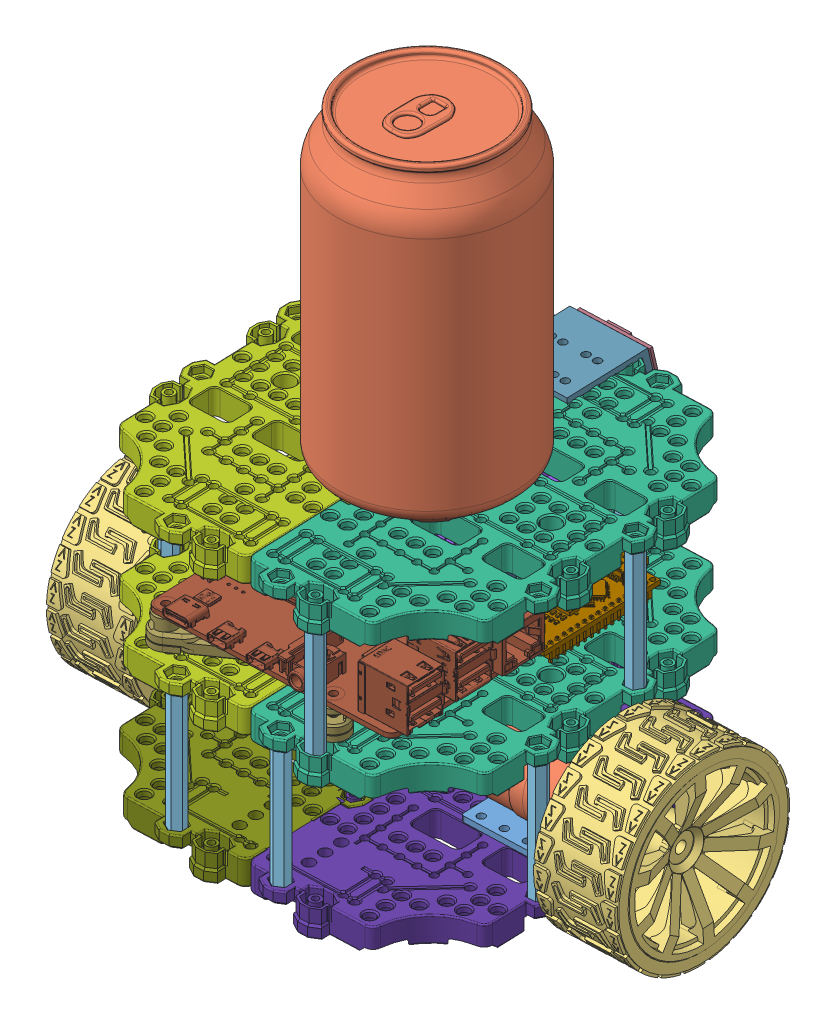
SolidWorks assembly BumperBotConveyor, configuration Default. Lengths in mm.
Overall size (200.73 230.35 157.69).
44 component instances, 20 part files, 117 mates.
Components (placement in the parent):
- motor_support-1: motor_support [Default] at (-39.885 107.5277 104.4569) x (-0.035505 0 -0.999369) z (0.999369 0 -0.035505) size (28 29 41)
- motor_support-2: motor_support [Default] at (97.5755 107.5277 99.5732) x (0.035505 0 0.999369) z (-0.999369 0 0.035505) size (28 29 41)
- JGA25-370-1: JGA25-370 [Default] at (52.3299 107.5277 101.1807) x (0.999369 0 -0.035505) z (0 -1 0) size (70.5 25.2 25.2)
- JGA25-370-2: JGA25-370 [Default] at (5.3607 107.5277 102.8494) x (-0.999369 0 0.035505) z (0 -1 0) size (70.5 25.2 25.2)
- wheel-1: wheel [Default] at (-18.4133 64.9311 67.753) x (0.033104 -0.361489 0.931789) z (-0.999369 0 0.035505) size (65.01 65.01 29)
- wheel_motor_adapter-1: wheel_motor_adapter [Default] at (-52.3777 107.532 104.885) x (0.034231 -0.265538 0.963493) z (-0.999369 0 0.035505) size (13.7 12 18.23)
- wheel-2: wheel [Default] at (76.6746 127.5563 152.3432) x (0.001314 -0.999315 0.036975) z (0.999369 0 -0.035505) size (65.01 65.01 29)
- wheel_motor_adapter-2: wheel_motor_adapter [Default] at (110.0677 107.5439 99.1304) x (-0.002274 -0.997947 -0.064012) z (0.999369 0 -0.035505) size (13.7 12 18.23)
- SUPPORT_HEX_M3_0XL45_FF-1: SUPPORT_HEX_M3_0XL45_FF [Default] at (50.5578 90.0277 37.2033) x (-0.5 0 0.866025) z (-0.866025 0 -0.5) size (5 45 5.77)
- SUPPORT_HEX_M3_0XL45_FF-6: SUPPORT_HEX_M3_0XL45_FF [Default] at (7.1327 90.0277 166.8268) x (0.255141 0 -0.966904) z (0.966904 0 0.255141) size (5 45 5.77)
- waffle_front_plate-3: waffle_front_plate [Default] at (28.8453 139.5277 102.0151) x (0.999369 0 -0.035505) z (0.035505 0 0.999369) size (73.55 9.85 137.55)
- waffle_rear_plate-2: waffle_rear_plate [Default] at (28.8453 139.5277 102.0151) x (-0.999369 0 0.035505) z (-0.035505 0 -0.999369) size (73.55 9.85 137.55)
- SUPPORT_HEX_M3_0XL45_FF-7: SUPPORT_HEX_M3_0XL45_FF [Default] at (2.588 87.5277 38.9075) x (0 0 -1) z (1 0 0) size (5 45 5.77)
- SUPPORT_HEX_M3_0XL45_FF-17: SUPPORT_HEX_M3_0XL45_FF [Default] at (-35.9665 135.0277 80.3025) x (0.866025 0 0.5) z (0.5 0 -0.866025) size (5 45 5.77)
- SUPPORT_HEX_M3_0XL45_FF-18: SUPPORT_HEX_M3_0XL45_FF [Default] at (93.657 135.0277 123.7276) x (0.866025 0 0.5) z (0.5 0 -0.866025) size (5 45 5.77)
- L298N-2: L298N [Default] at (11.4909 149.5277 70.3617) x (0.999369 0 -0.035505) z (0.035505 0 0.999369) size (50 22 50)
- Arduino Nano-2: Arduino Nano [Default] at (42.2606 141.5277 53.4388) x (0.035505 0 0.999369) z (0 1 0) size (44.28 18 13.68)
- board_bracket_small-1: board_bracket_small [Default] at (33.6312 139.5277 47.5214) x (0.998944 0 -0.045937) z (0.045937 0 0.998944) size (37.82 10 10.43)
- board_bracket_small-2: board_bracket_small [Default] at (-10.6494 139.5277 93.2019) x (0.065728 0 0.997838) z (-0.997838 0 0.065728) size (37.82 10 10.43)
- board_bracket_small-3: board_bracket_small [Default] at (35.1962 139.5277 91.5731) x (0.107735 0 0.99418) z (-0.99418 0 0.107735) size (37.82 10 10.43)
- SUPPORT_HEX_M3_0XL45_FF-20: SUPPORT_HEX_M3_0XL45_FF [Default] at (-34.2623 179.8277 128.2723) x (0.530433 0 0.847727) z (0.847727 0 -0.530433) size (5 45 5.77)
- SUPPORT_HEX_M3_0XL45_FF-21: SUPPORT_HEX_M3_0XL45_FF [Default] at (14.5805 182.0277 38.4815) x (-0.999369 0 0.035505) z (0.035505 0 0.999369) size (5 45 5.77)
- SUPPORT_HEX_M3_0XL45_FF-22: SUPPORT_HEX_M3_0XL45_FF [Default] at (-35.5405 179.8277 92.295) x (-0.468936 0 0.883232) z (0.883232 0 0.468936) size (5 45 5.77)
- SUPPORT_HEX_M3_0XL45_FF-23: SUPPORT_HEX_M3_0XL45_FF [Default] at (38.5654 179.8277 37.6293) x (0.035505 0 0.999369) z (0.999369 0 -0.035505) size (5 45 5.77)
- SUPPORT_HEX_M3_0XL45_FF-25: SUPPORT_HEX_M3_0XL45_FF [Default] at (43.11 135.0277 165.5486) x (1 0 0) z (0 0 -1) size (5 45 5.77)
- SUPPORT_HEX_M3_0XL45_FF-26: SUPPORT_HEX_M3_0XL45_FF [Default] at (55.1025 179.8277 165.1226) x (0.883232 0 0.468936) z (0.468936 0 -0.883232) size (5 45 5.77)
- SUPPORT_HEX_M3_0XL45_FF-27: SUPPORT_HEX_M3_0XL45_FF [Default] at (92.3788 182.0277 87.7503) x (0.035505 0 0.999369) z (0.999369 0 -0.035505) size (5 45 5.77)
- Raspberry Pi 4 Model B-3: Raspberry Pi 4 Model B [Default] at (149.9317 65.3277 125.8391) x (0.999369 0 -0.035505) z (0 1 0) size (89.07 58.45 20.84)
- board_bracket-5: board_bracket [Default] at (53.2833 139.5277 156.9085) x (0.727355 0 0.686261) z (-0.686261 0 0.727355) size (37.82 10 10.2)
- board_bracket-6: board_bracket [Default] at (51.5435 139.5277 107.9394) x (-0.255641 0 -0.966772) z (0.966772 0 -0.255641) size (37.82 10 10.2)
- board_bracket-7: board_bracket [Default] at (-4.6801 139.5277 158.9678) x (-0.81984 0 0.572593) z (-0.572593 0 -0.81984) size (37.82 10 10.2)
- board_bracket-8: board_bracket [Default] at (-6.4199 139.5277 109.9987) x (-0.570741 0 -0.82113) z (0.82113 0 -0.570741) size (37.82 10 10.2)
- waffle_rear_plate-3: waffle_rear_plate [Default] at (28.8453 186.5277 102.0151) x (-0.999369 0 0.035505) z (-0.035505 0 -0.999369) size (73.55 9.85 137.55)
- waffle_front_plate-4: waffle_front_plate [Default] at (28.8453 186.8277 102.0151) x (0.999369 0 -0.035505) z (0.035505 0 0.999369) size (73.55 9.85 137.55)
- RPi cam Rev 1.3-1: RPi cam Rev 1.3 [Výchozí] at (26.1362 175.4612 25.7618) x (0.999369 0 -0.035505) z (-0.03451 0.235171 -0.971341) size (25.2 33.1 8.7)
- camera_stand_reversed-1: camera_stand_reversed [Default] at (40.8891 188.5277 60.7879) x (0.035505 0 0.999369) z (-0.999369 0 0.035505) size (34.33 18.42 27)
- MPU_6050-1: MPU_6050 [Default] at (29.2409 176.3277 107.5422) x (1 0 0) z (0 -1 0) size (20.5 16 3)
- waffle_rear_base_plate-1: waffle_rear_base_plate [Default] at (28.8453 92.5277 102.0151) x (-0.999369 0 0.035505) z (-0.035505 0 -0.999369) size (73.55 9.85 137.55)
- waffle_front_base_plate-1: waffle_front_base_plate [Default] at (28.8453 92.5277 102.0151) x (0.999369 0 -0.035505) z (0.035505 0 0.999369) size (73.55 9.85 137.55)
- waffle_caster_support-4: waffle_caster_support [Default] at (30.5335 87.0277 149.5351) x (-0.999369 0 0.035505) z (0.035505 0 0.999369) size (30 8.25 18.16)
- waffle_caster_support-5: waffle_caster_support [Default] at (27.157 87.0277 54.495) x (-0.999369 0 0.035505) z (0.035505 0 0.999369) size (30 8.25 18.16)
- waffle_caster_ball-4: waffle_caster_ball [Default] at (30.5335 83.1652 149.5351) size (9.53 9.53 9.53)
- waffle_caster_ball-5: waffle_caster_ball [Default] at (27.157 83.1652 54.495) size (9.53 9.53 9.53)
- coke-1: coke [Défaut] at (47.9029 239.3343 101.9085) size (64.24 111.99 64.24)
Mates (geometry in assembly coordinates):
- Coincident21: coincident anti-aligned: plane of motor_support-2 through (95.5768 107.5277 99.6442) normal (-0.999369 0 0.035505); plane of JGA25-370-1 through (96.0206 107.5277 112.1363) normal (0.999369 0 -0.035505)
- Concentric7: concentric aligned: circle of motor_support-2; circle of JGA25-370-1
- Concentric8: concentric aligned: cylinder of motor_support-2 through (95.275 107.5277 91.1496) axis (0.999369 0 -0.035505) radius 1.25; cylinder of JGA25-370-1 through (90.2781 107.5277 91.3271) axis (0.999369 0 -0.035505) radius 1.25
- Coincident22: coincident anti-aligned: plane of motor_support-1 through (-37.8863 107.5277 104.3859) normal (0.999369 0 -0.035505); plane of JGA25-370-2 through (-38.3301 107.5277 91.8938) normal (-0.999369 0 0.035505)
- Concentric9: concentric aligned: circle of motor_support-1; circle of JGA25-370-2
- Concentric10: concentric anti-aligned: circle of motor_support-1; circle of JGA25-370-2
- Coincident24: coincident anti-aligned: plane of wheel-1 through (-58.4359 114.2363 103.3532) normal (-0.009428 -0.964101 -0.26537); plane of wheel_motor_adapter-1 through (-58.1987 112.3966 110.0284) normal (0.009428 0.964101 0.26537)
- Coincident25: coincident anti-aligned: plane of wheel-1 through (-58.1367 105.6921 111.7739) normal (-0.024931 0.712013 -0.701724); plane of wheel_motor_adapter-1 through (-58.3119 100.8274 106.844) normal (0.024931 -0.712013 0.701724)
- Coincident26: coincident anti-aligned: plane of wheel-1 through (-58.3739 107.5318 105.0986) normal (0.999369 0 -0.035505); plane of wheel_motor_adapter-1 through (-58.3739 107.532 105.0981) normal (-0.999369 0 0.035505)
- Concentric11: concentric aligned: cylinder of JGA25-370-2 through (-50.3784 107.5277 104.8297) axis (0.999369 0 -0.035505) radius 1.95; cylinder of wheel_motor_adapter-1 through (-52.3771 107.5277 104.9007) axis (0.999369 0 -0.035505) radius 3
- Coincident30: coincident anti-aligned: plane of wheel-2 through (115.8592 111.3847 93.1552) normal (0.035432 -0.064052 0.997317); plane of wheel_motor_adapter-2 through (115.8434 104.4707 92.7117) normal (-0.035432 0.064052 -0.997317)
- Coincident31: coincident anti-aligned: plane of wheel-2 through (115.8434 104.4707 92.7117) normal (0.019686 0.832221 0.554094); plane of wheel_motor_adapter-2 through (116.0481 100.6294 98.4739) normal (-0.019686 -0.832221 -0.554094)
- Coincident32: coincident anti-aligned: plane of wheel-2 through (116.0639 107.5434 98.9174) normal (-0.999369 0 0.035505); plane of wheel_motor_adapter-2 through (116.0639 107.5439 98.9174) normal (0.999369 0 -0.035505)
- Concentric16: concentric aligned: cylinder of JGA25-370-1 through (108.0689 107.5277 99.2004) axis (-0.999369 0 0.035505) radius 1.95; cylinder of wheel_motor_adapter-2 through (110.0676 107.5277 99.1294) axis (-0.999369 0 0.035505) radius 3
- Coincident33: coincident anti-aligned: plane of JGA25-370-1 through (98.0752 107.5277 99.5555) normal (0.999369 0 -0.035505); plane of wheel_motor_adapter-2 through (98.0752 107.5439 99.5565) normal (-0.999369 0 0.035505)
- Coincident34: coincident anti-aligned: plane of JGA25-370-2 through (-40.3847 107.5277 104.4746) normal (-0.999369 0 0.035505); plane of wheel_motor_adapter-1 through (-40.3852 107.532 104.459) normal (0.999369 0 -0.035505)
- Coincident72: coincident anti-aligned: plane of SUPPORT_HEX_M3_0XL45_FF-1 through (50.5578 135.0277 37.2033) normal (0 1 0); plane of waffle_front_plate-3 through (28.8453 135.0277 102.0151) normal (0 -1 0)
- Concentric28: concentric anti-aligned: cylinder of SUPPORT_HEX_M3_0XL45_FF-1 through (50.5578 123.739 37.2033) axis (0 -1 0) radius 1.25; cylinder of waffle_front_plate-3 through (50.5578 129.1327 37.2033) axis (0 1 0) radius 1.6
- Concentric30: concentric anti-aligned: cylinder of SUPPORT_HEX_M3_0XL45_FF-6 through (7.1327 123.739 166.8268) axis (0 -1 0) radius 1.25; cylinder of waffle_rear_plate-2 through (7.1327 129.1327 166.8268) axis (0 1 0) radius 1.6
- Coincident74: coincident anti-aligned: plane of SUPPORT_HEX_M3_0XL45_FF-6 through (7.1327 135.0277 166.8268) normal (0 1 0); plane of waffle_rear_plate-2 through (28.8453 135.0277 102.0151) normal (0 -1 0)
- Concentric33: concentric aligned: circle of waffle_rear_plate-2; circle of SUPPORT_HEX_M3_0XL45_FF-7
- Parallel33: parallel aligned: plane of waffle_rear_plate-2 through (14.411 137.2777 33.711) normal (-0.035505 0 -0.999369); plane of L298N-2 through (-14.381 150.5277 46.2651) normal (-0.035505 0 -0.999369)
- Parallel34: parallel anti-aligned: plane of waffle_front_plate-3 through (28.8453 139.5277 102.0151) normal (0 1 0); plane of L298N-2 through (11.4909 149.5277 70.3617) normal (0 -1 0)
- Parallel35: parallel aligned: plane of waffle_front_plate-3 through (90.5326 139.5277 35.7831) normal (-0.035505 0 -0.999369); plane of Arduino Nano-2 through (70.9901 145.6677 57.4663) normal (-0.035505 0 -0.999369)
- Parallel36: parallel anti-aligned: plane of waffle_front_plate-3 through (28.8453 139.5277 102.0151) normal (0 1 0); plane of Arduino Nano-2 through (54.5159 144.0677 61.864) normal (0 -1 0)
- Concentric72: concentric aligned: cylinder of L298N-2 through (33.6312 149.5277 47.5214) axis (0 1 0) radius 1.5; circle of board_bracket_small-1
- Coincident123: coincident anti-aligned: plane of L298N-2 through (11.4909 149.5277 70.3617) normal (0 -1 0); plane of board_bracket_small-1 through (33.6312 149.5277 47.5214) normal (0 1 0)
- Coincident124: coincident anti-aligned: plane of waffle_rear_plate-2 through (28.8453 139.5277 102.0151) normal (0 1 0); plane of board_bracket_small-1 through (5.9412 139.5277 48.7947) normal (0 -1 0)
- Concentric73: concentric anti-aligned: cylinder of waffle_rear_plate-2 through (5.9412 139.5277 48.7947) axis (0 -1 0) radius 2.5; cylinder of board_bracket_small-1 through (5.9412 126.4917 48.7947) axis (0 1 0) radius 5
- Lock5: lock: unknown of waffle_front_plate-3; unknown of board_bracket_small-1
- Concentric75: concentric aligned: circle of L298N-2; cylinder of board_bracket_small-2 through (-10.6494 149.5277 93.2019) axis (0 1 0) radius 1
- Coincident125: coincident anti-aligned: plane of L298N-2 through (11.4909 149.5277 70.3617) normal (0 -1 0); plane of board_bracket_small-2 through (-10.6494 149.5277 93.2019) normal (0 1 0)
- Lock6: lock: unknown of waffle_rear_plate-2; unknown of board_bracket_small-2
- Concentric78: concentric aligned: cylinder of L298N-2 through (35.1962 149.5277 91.5731) axis (0 1 0) radius 1.5; cylinder of board_bracket_small-3 through (35.1962 149.5277 91.5731) axis (0 1 0) radius 1
- Coincident126: coincident anti-aligned: plane of L298N-2 through (11.4909 149.5277 70.3617) normal (0 -1 0); plane of board_bracket_small-3 through (35.1962 149.5277 91.5731) normal (0 1 0)
- Lock7: lock: unknown of waffle_front_plate-3; unknown of board_bracket_small-3
- Concentric81: concentric aligned: circle of waffle_rear_plate-2; cylinder of SUPPORT_HEX_M3_0XL45_FF-20 through (-34.2623 146.1163 128.2723) axis (0 1 0) radius 1.25
- Coincident129: coincident anti-aligned: plane of waffle_rear_plate-2 through (28.8453 134.8277 102.0151) normal (0 1 0); plane of SUPPORT_HEX_M3_0XL45_FF-20 through (-34.2623 134.8277 128.2723) normal (0 -1 0)
- Parallel44: parallel aligned: plane of waffle_rear_plate-2 through (-38.4889 139.5277 126.8502) normal (-0.999369 0 0.035505); plane of SUPPORT_HEX_M3_0XL45_FF-20 through (-36.7094 179.8277 129.8035) normal (-0.999369 0 0.035505)
- Concentric82: concentric aligned: cylinder of waffle_rear_plate-2 through (14.5805 129.1327 38.4815) axis (0 1 0) radius 1.6; cylinder of SUPPORT_HEX_M3_0XL45_FF-21 through (14.5805 148.3163 38.4815) axis (0 1 0) radius 1.25
- Coincident131: coincident anti-aligned: plane of waffle_rear_plate-2 through (28.8453 137.0277 102.0151) normal (0 1 0); plane of SUPPORT_HEX_M3_0XL45_FF-21 through (14.5805 137.0277 38.4815) normal (0 -1 0)
- Concentric83: concentric anti-aligned: cylinder of waffle_rear_plate-2 through (-35.5405 139.5277 92.295) axis (0 1 0) radius 1.2; circle of SUPPORT_HEX_M3_0XL45_FF-22
- Coincident133: coincident anti-aligned: plane of waffle_rear_plate-2 through (28.8453 134.8277 102.0151) normal (0 1 0); plane of SUPPORT_HEX_M3_0XL45_FF-22 through (-35.5405 134.8277 92.295) normal (0 -1 0)
- Parallel46: parallel aligned: plane of waffle_rear_plate-2 through (-39.7671 139.5277 90.8729) normal (-0.999369 0 0.035505); plane of SUPPORT_HEX_M3_0XL45_FF-22 through (-37.9876 179.8277 93.8262) normal (-0.999369 0 0.035505)
- Concentric84: concentric aligned: cylinder of waffle_front_plate-3 through (38.5654 139.5277 37.6293) axis (0 1 0) radius 1.2; cylinder of SUPPORT_HEX_M3_0XL45_FF-23 through (38.5654 146.1163 37.6293) axis (0 1 0) radius 1.25
- Coincident135: coincident anti-aligned: plane of waffle_front_plate-3 through (28.8453 134.8277 102.0151) normal (0 1 0); plane of SUPPORT_HEX_M3_0XL45_FF-23 through (38.5654 134.8277 37.6293) normal (0 -1 0)
- Parallel47: parallel aligned: plane of waffle_front_plate-3 through (39.9875 139.5277 33.4027) normal (-0.035505 0 -0.999369); plane of SUPPORT_HEX_M3_0XL45_FF-23 through (37.0341 179.8277 35.1822) normal (-0.035505 0 -0.999369)
- Concentric87: concentric aligned: cylinder of waffle_front_plate-3 through (55.1025 139.5277 165.1226) axis (0 1 0) radius 1.2; cylinder of SUPPORT_HEX_M3_0XL45_FF-26 through (55.1025 146.1163 165.1226) axis (0 1 0) radius 1.25
- Coincident141: coincident anti-aligned: plane of waffle_front_plate-3 through (28.8453 134.8277 102.0151) normal (0 1 0); plane of SUPPORT_HEX_M3_0XL45_FF-26 through (55.1025 134.8277 165.1226) normal (0 -1 0)
- Parallel50: parallel aligned: plane of waffle_front_plate-3 through (53.6804 139.5277 169.3492) normal (0.035505 0 0.999369); plane of SUPPORT_HEX_M3_0XL45_FF-26 through (56.6337 179.8277 167.5697) normal (0.035505 0 0.999369)
- Concentric88: concentric aligned: circle of waffle_front_plate-3; cylinder of SUPPORT_HEX_M3_0XL45_FF-27 through (92.3788 148.3163 87.7503) axis (0 1 0) radius 1.25
- Coincident143: coincident anti-aligned: plane of waffle_front_plate-3 through (28.8453 137.0277 102.0151) normal (0 1 0); plane of SUPPORT_HEX_M3_0XL45_FF-27 through (92.3788 137.0277 87.7503) normal (0 -1 0)
- Parallel51: parallel aligned: plane of waffle_front_plate-3 through (95.4413 139.5277 92.6446) normal (0.883232 0 0.468936); plane of SUPPORT_HEX_M3_0XL45_FF-27 through (95.2638 182.0277 87.6478) normal (0.883232 0 0.468936)
- Parallel52: parallel anti-aligned: plane of waffle_rear_plate-2 through (28.8453 139.5277 102.0151) normal (0 1 0); plane of Raspberry Pi 4 Model B-3 through (-5.1621 149.5277 159.4852) normal (0 -1 0)
- Parallel53: parallel aligned: plane of waffle_front_plate-3 through (31.1176 139.5277 165.9747) normal (0.035505 0 0.999369); plane of Raspberry Pi 4 Model B-3 through (-5.0556 151.1277 162.4833) normal (0.035505 0 0.999369)
- Parallel54: parallel aligned: plane of waffle_front_plate-3 through (95.0773 139.5277 163.7024) normal (0.999369 0 -0.035505); plane of Raspberry Pi 4 Model B-3 through (76.7862 151.1277 156.5738) normal (0.999369 0 -0.035505)
- Coincident148: coincident aligned: plane of waffle_front_plate-3 through (54.933 137.2777 160.3521) normal (0.035505 0 0.999369); plane of Raspberry Pi 4 Model B-3 through (-5.0556 151.1277 162.4833) normal (0.035505 0 0.999369)
- Concentric90: concentric anti-aligned: cylinder of Raspberry Pi 4 Model B-3 through (53.2833 149.4277 156.9085) axis (0 1 0) radius 1.35; cylinder of board_bracket-5 through (53.2833 150.5277 156.9085) axis (0 -1 0) radius 2
- Coincident149: coincident anti-aligned: plane of Raspberry Pi 4 Model B-3 through (-5.1621 149.5277 159.4852) normal (0 -1 0); plane of board_bracket-5 through (46.2152 149.5277 157.1139) normal (0 1 0)
- Coincident150: coincident anti-aligned: plane of waffle_front_plate-3 through (28.8453 139.5277 102.0151) normal (0 1 0); plane of board_bracket-5 through (47.6699 139.5277 158.4865) normal (0 -1 0)
- Concentric91: concentric aligned: cylinder of waffle_front_plate-3 through (33.1216 138.7277 137.8858) axis (0 1 0) radius 2; cylinder of board_bracket-5 through (33.1216 126.4917 137.8858) axis (0 1 0) radius 5
- Concentric92: concentric anti-aligned: cylinder of Raspberry Pi 4 Model B-3 through (51.5435 149.4277 107.9394) axis (0 1 0) radius 1.35; cylinder of board_bracket-6 through (51.5435 150.5277 107.9394) axis (0 -1 0) radius 2
- Coincident151: coincident anti-aligned: plane of Raspberry Pi 4 Model B-3 through (-5.1621 149.5277 159.4852) normal (0 -1 0); plane of board_bracket-6 through (57.6556 149.5277 111.495) normal (0 1 0)
- Lock8: lock: unknown of waffle_front_plate-3; unknown of board_bracket-6
- Concentric94: concentric anti-aligned: cylinder of Raspberry Pi 4 Model B-3 through (-4.6801 149.4277 158.9678) axis (0 1 0) radius 1.35; cylinder of board_bracket-7 through (-4.6801 150.5277 158.9678) axis (0 -1 0) radius 2
- Coincident152: coincident anti-aligned: plane of Raspberry Pi 4 Model B-3 through (-5.1621 149.5277 159.4852) normal (0 -1 0); plane of board_bracket-7 through (-3.4439 149.5277 152.0056) normal (0 1 0)
- Lock9: lock: unknown of waffle_rear_plate-2; unknown of board_bracket-7
- Concentric96: concentric anti-aligned: cylinder of Raspberry Pi 4 Model B-3 through (-6.4199 149.4277 109.9987) axis (0 1 0) radius 1.3; cylinder of board_bracket-8 through (-6.4199 150.5277 109.9987) axis (0 -1 0) radius 2
- Coincident153: coincident anti-aligned: plane of Raspberry Pi 4 Model B-3 through (-5.1621 149.5277 159.4852) normal (0 -1 0); plane of board_bracket-8 through (0.5395 149.5277 111.2506) normal (0 1 0)
- Lock10: lock: unknown of waffle_rear_plate-2; unknown of board_bracket-8
- Parallel58: parallel anti-aligned: plane of waffle_rear_plate-2 through (17.3213 139.5277 36.7665) normal (-0.468936 0 0.883232); plane of SUPPORT_HEX_M3_0XL45_FF-21 through (14.478 182.0277 35.5965) normal (0.468936 0 -0.883232)
- Concentric98: concentric aligned: cylinder of SUPPORT_HEX_M3_0XL45_FF-21 through (14.5805 170.739 38.4815) axis (0 1 0) radius 1.25; cylinder of waffle_rear_plate-3 through (14.5805 176.1327 38.4815) axis (0 1 0) radius 1.6
- Coincident156: coincident anti-aligned: plane of SUPPORT_HEX_M3_0XL45_FF-21 through (14.5805 182.0277 38.4815) normal (0 1 0); plane of waffle_rear_plate-3 through (28.8453 182.0277 102.0151) normal (0 -1 0)
- Concentric99: concentric aligned: cylinder of SUPPORT_HEX_M3_0XL45_FF-20 through (-34.2623 168.539 128.2723) axis (0 1 0) radius 1.25; cylinder of waffle_rear_plate-3 through (-34.2623 186.5277 128.2723) axis (0 1 0) radius 1.2
- Concentric100: concentric aligned: cylinder of SUPPORT_HEX_M3_0XL45_FF-23 through (38.5654 168.539 37.6293) axis (0 1 0) radius 1.25; cylinder of waffle_front_plate-4 through (38.5654 176.4327 37.6293) axis (0 1 0) radius 1.6
- Coincident157: coincident anti-aligned: plane of SUPPORT_HEX_M3_0XL45_FF-23 through (38.5654 179.8277 37.6293) normal (0 1 0); plane of waffle_front_plate-4 through (28.8453 179.8277 102.0151) normal (0 -1 0)
- Concentric101: concentric aligned: cylinder of SUPPORT_HEX_M3_0XL45_FF-26 through (55.1025 168.539 165.1226) axis (0 1 0) radius 1.25; cylinder of waffle_front_plate-4 through (55.1025 186.8277 165.1226) axis (0 1 0) radius 1.2
- Concentric114: concentric aligned: cylinder of waffle_front_plate-4 through (34.7809 176.4327 43.7676) axis (0 1 0) radius 1.35; cylinder of camera_stand_reversed-1 through (34.7809 168.5277 43.7676) axis (0 1 0) radius 1.35
- Concentric115: concentric anti-aligned: cylinder of waffle_rear_plate-3 through (19.2171 176.1327 56.3281) axis (0 -1 0) radius 1.35; cylinder of camera_stand_reversed-1 through (19.2171 168.5277 56.3281) axis (0 1 0) radius 1.35
- Coincident171: coincident anti-aligned: plane of waffle_rear_plate-3 through (28.8453 186.5277 102.0151) normal (0 1 0); plane of camera_stand_reversed-1 through (13.9061 186.5277 61.7466) normal (0 -1 0)
- Coincident172: coincident anti-aligned: plane of RPi cam Rev 1.3-1 through (26.2155 174.9203 27.9959) normal (0.03451 -0.235171 0.971341); plane of camera_stand_reversed-1 through (12.6871 170.6246 27.4365) normal (-0.03451 0.235171 -0.971341)
- Concentric116: concentric aligned: cylinder of RPi cam Rev 1.3-1 through (36.7492 185.14 28.7575) axis (-0.03451 0.235171 -0.971341) radius 1.05; cylinder of camera_stand_reversed-1 through (37.4843 180.1308 49.4471) axis (-0.03451 0.235171 -0.971341) radius 1
- Concentric117: concentric aligned: cylinder of RPi cam Rev 1.3-1 through (15.6597 173.1849 26.6124) axis (-0.03451 0.235171 -0.971341) radius 1.05; cylinder of camera_stand_reversed-1 through (16.3948 168.1758 47.3019) axis (-0.03451 0.235171 -0.971341) radius 1
- Coincident173: coincident anti-aligned: plane of waffle_front_plate-4 through (28.8453 177.8277 102.0151) normal (0 -1 0); plane of MPU_6050-1 through (29.2409 177.8277 107.5422) normal (0 1 0)
- Concentric119: concentric aligned: circle of waffle_rear_plate-3; cylinder of MPU_6050-1 through (21.2409 176.3277 113.2922) axis (0 1 0) radius 1.5
- Concentric122: concentric anti-aligned: cylinder of waffle_front_plate-3 through (43.11 129.1327 165.5486) axis (0 1 0) radius 1.6; circle of SUPPORT_HEX_M3_0XL45_FF-25
- Concentric124: concentric anti-aligned: cylinder of SUPPORT_HEX_M3_0XL45_FF-6 through (7.1327 101.3163 166.8268) axis (0 -1 0) radius 1.25; cylinder of waffle_rear_base_plate-1 through (7.1327 82.1327 166.8268) axis (0 1 0) radius 1.6
- Coincident178: coincident anti-aligned: plane of SUPPORT_HEX_M3_0XL45_FF-6 through (7.1327 90.0277 166.8268) normal (0 -1 0); plane of waffle_rear_base_plate-1 through (28.8453 90.0277 102.0151) normal (0 1 0)
- Concentric125: concentric anti-aligned: cylinder of SUPPORT_HEX_M3_0XL45_FF-7 through (2.588 98.8163 38.9075) axis (0 -1 0) radius 1.25; cylinder of waffle_rear_base_plate-1 through (2.588 92.5277 38.9075) axis (0 1 0) radius 1.2
- Coincident179: coincident anti-aligned: plane of motor_support-1 through (-38.3833 92.5277 90.3947) normal (0 -1 0); plane of waffle_rear_base_plate-1 through (28.8453 92.5277 102.0151) normal (0 1 0)
- Coincident180: coincident anti-aligned: circle of motor_support-1; cylinder of waffle_rear_base_plate-1 through (-2.744 83.5277 114.1443) axis (0 -1 0) radius 1.35
- Concentric126: concentric anti-aligned: cylinder of motor_support-1 through (-27.51 77.5277 93.0103) axis (0 1 0) radius 1.35; cylinder of waffle_rear_base_plate-1 through (-27.51 83.5277 93.0103) axis (0 -1 0) radius 1.35
- Coincident181: coincident anti-aligned: plane of waffle_front_plate-3 through (28.8453 135.0277 102.0151) normal (0 -1 0); plane of SUPPORT_HEX_M3_0XL45_FF-25 through (43.11 135.0277 165.5486) normal (0 1 0)
- Coincident182: coincident anti-aligned: plane of waffle_front_plate-3 through (28.8453 135.0277 102.0151) normal (0 -1 0); plane of SUPPORT_HEX_M3_0XL45_FF-18 through (93.657 135.0277 123.7276) normal (0 1 0)
- Coincident184: coincident anti-aligned: plane of waffle_rear_plate-2 through (28.8453 132.5277 102.0151) normal (0 -1 0); plane of SUPPORT_HEX_M3_0XL45_FF-7 through (2.588 132.5277 38.9075) normal (0 1 0)
- Coincident185: coincident anti-aligned: plane of waffle_rear_plate-2 through (28.8453 135.0277 102.0151) normal (0 -1 0); plane of SUPPORT_HEX_M3_0XL45_FF-17 through (-35.9665 135.0277 80.3025) normal (0 1 0)
- Concentric127: concentric anti-aligned: cylinder of waffle_front_plate-3 through (93.657 129.1327 123.7276) axis (0 1 0) radius 1.6; circle of SUPPORT_HEX_M3_0XL45_FF-18
- Concentric128: concentric anti-aligned: circle of waffle_rear_plate-2; cylinder of SUPPORT_HEX_M3_0XL45_FF-17 through (-35.9665 123.739 80.3025) axis (0 1 0) radius 1.25
- Concentric129: concentric aligned: cylinder of SUPPORT_HEX_M3_0XL45_FF-17 through (-35.9665 123.739 80.3025) axis (0 1 0) radius 1.25; cylinder of waffle_rear_base_plate-1 through (-35.9665 82.1327 80.3025) axis (0 1 0) radius 1.6
- Coincident186: coincident anti-aligned: plane of waffle_front_plate-3 through (28.8453 139.5277 102.0151) normal (0 1 0); plane of Arduino Nano-2 through (54.5159 139.5277 61.864) normal (0 -1 0)
- Coincident187: coincident aligned: plane of waffle_front_plate-3 through (71.6656 139.5277 76.4786) normal (0.999369 0 -0.035505); plane of Arduino Nano-2 through (70.9901 145.6677 57.4663) normal (0.999369 0 -0.035505)
- Concentric130: concentric anti-aligned: circle of waffle_rear_base_plate-1; cylinder of waffle_front_base_plate-1 through (29.6974 92.5277 125.9999) axis (0 1 0) radius 1.2
- Concentric131: concentric aligned: cylinder of waffle_rear_base_plate-1 through (27.9931 92.5277 78.0302) axis (0 1 0) radius 1.2; cylinder of waffle_front_base_plate-1 through (27.9931 82.1327 78.0302) axis (0 1 0) radius 1.6
- Coincident189: coincident aligned: plane of waffle_rear_base_plate-1 through (18.7541 88.5277 155.9574) normal (0 -1 0); plane of waffle_front_base_plate-1 through (42.739 88.5277 155.1052) normal (0 -1 0)
- Coincident190: coincident anti-aligned: plane of motor_support-2 through (96.0739 92.5277 113.6354) normal (0 -1 0); plane of waffle_front_base_plate-1 through (28.8453 92.5277 102.0151) normal (0 1 0)
- Concentric132: concentric anti-aligned: cylinder of motor_support-2 through (61.2156 77.5277 111.8719) axis (0 1 0) radius 1.35; cylinder of waffle_front_base_plate-1 through (61.2156 83.5277 111.8719) axis (0 -1 0) radius 1.35
- Concentric133: concentric anti-aligned: cylinder of motor_support-2 through (84.4194 77.5277 89.0337) axis (0 1 0) radius 1.35; cylinder of waffle_front_base_plate-1 through (84.4194 83.5277 89.0337) axis (0 -1 0) radius 1.35
- Coincident191: coincident anti-aligned: plane of waffle_front_base_plate-1 through (42.739 88.5277 155.1052) normal (0 -1 0); plane of waffle_caster_support-4 through (30.5335 88.5277 149.5351) normal (0 1 0)
- Concentric134: concentric anti-aligned: cylinder of waffle_front_base_plate-1 through (42.3129 92.5277 143.1128) axis (0 -1 0) radius 2; cylinder of waffle_caster_support-4 through (42.3129 87.7277 143.1128) axis (0 1 0) radius 2.01
- Coincident192: coincident anti-aligned: plane of waffle_rear_base_plate-1 through (14.9515 88.5277 48.9249) normal (0 -1 0); plane of waffle_caster_support-5 through (27.157 88.5277 54.495) normal (0 1 0)
- Concentric140: concentric anti-aligned: cylinder of waffle_rear_base_plate-1 through (15.3776 92.5277 60.9173) axis (0 -1 0) radius 2; cylinder of waffle_caster_support-5 through (15.3776 87.7277 60.9173) axis (0 1 0) radius 2.01
- Concentric141: concentric anti-aligned: cylinder of waffle_front_base_plate-1 through (38.9364 92.5277 48.0728) axis (0 -1 0) radius 2; cylinder of waffle_caster_support-5 through (38.9364 87.7277 48.0728) axis (0 1 0) radius 2.01
- Concentric144: concentric anti-aligned: cylinder of waffle_front_base_plate-1 through (42.739 92.5277 155.1052) axis (0 -1 0) radius 2; cylinder of waffle_caster_support-4 through (42.739 87.7277 155.1052) axis (0 1 0) radius 2.01
- Concentric145: concentric: sphere of waffle_caster_support-4; sphere of waffle_caster_ball-4
- Concentric146: concentric: sphere of waffle_caster_support-5; sphere of waffle_caster_ball-5
- Tangent1: tangent: plane of waffle_front_plate-4 through (28.8453 186.8277 102.0151) normal (0 1 0); torus of coke-1
- Concentric147: concentric aligned: circle of waffle_front_plate-4; circle of coke-1
